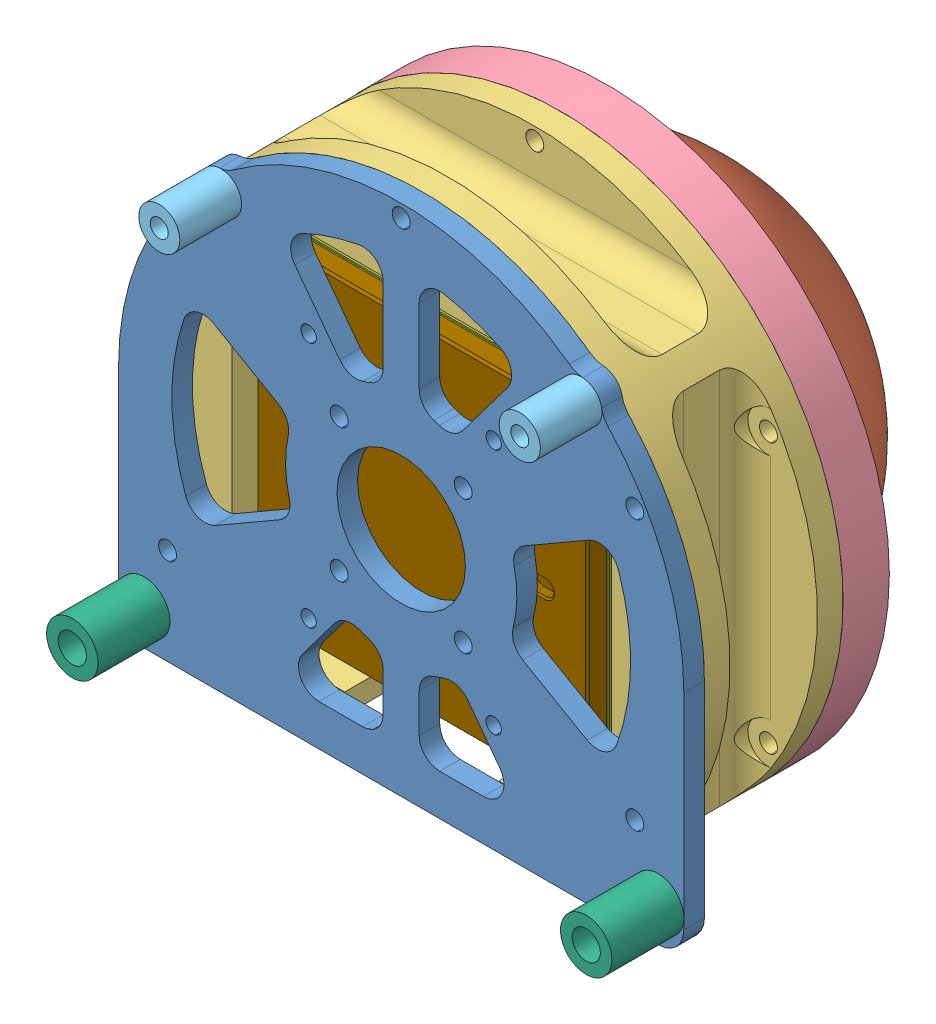
SolidWorks assembly MID保护安装版装配体, configuration 默认. Lengths in mm.
Overall size (1862.57 1865.26 855.73).
19 component instances, 15 part files, 20 mates.
Components (placement in the parent):
- IMU安装板11111-1: IMU安装板11111 [默认] at (-66.2823 -28.2156 -2) size (110 100 4)
- MID_360罩子-1: MID_360罩子 [默认] at (-66.2823 19.7844 -29) x (0.511073 -0.859537 0) z (0.859537 0.511073 0) size (99.6 45 99.6)
- MID保护罩支撑2222-1: MID保护罩支撑2222 [默认] at (-66.2823 -28.2156 -29) size (110 95.89 27)
- 舱盖固定环-1: 舱盖固定环 [默认] at (-66.2823 19.7844 -29) x (-1 0 0) z (0 0 -1) size (110 110 9)
- 支撑短-1: 支撑短 [默认] at (-31.2083 59.0344 2) x (-0.318059 -0.948071 0) z (0 0 1) size (8 8 12)
- 支撑长-1: 支撑长 [默认] at (-16.2823 -18.2156 2) x (-0.53223 0.8466 0) z (0 0 1) size (10 10 14)
- 支撑短-2: 支撑短 [默认] at (-101.3564 59.0344 2) x (0.71117 0.70302 0) z (0 0 1) size (8 8 12)
- 支撑长-2: 支撑长 [默认] at (-116.2823 -18.2156 2) x (0.671555 -0.740955 0) z (0 0 1) size (10 10 14)
- mid-360-fov-asm (1)-1: mid-360-fov-asm (1) [默认] at (-66.2823 19.7844 -27.9171) x (0 -1 0) z (1 0 0) size (1865.26 855.73 1862.57)
  - MID-360_4_ASM_2_ASM-1: MID-360_4_ASM_2_ASM [默认] at origin size (72.74 69.7 66.83)
    - MID-360_4_ASM_2_ASM-1: MID-360_4_ASM_2_ASM [默认] at origin size (71.74 36.3 66.83)
    - MID-360_4_1_1-1: MID-360_4_1_1 [默认] at origin size (52.18 60.17 55.44)
    - MID-360_4_2_1-1: MID-360_4_2_1 [默认] at origin size (64.79 8.1 64.79)
    - MID-360_4_3_2-1: MID-360_4_3_2 [默认] at origin size (13.8 16 22)
    - MID-360_4_4_1-1: MID-360_4_4_1 [默认] at origin size (0.41 0.13 0.13)
    - MID-360_4_5_1-1: MID-360_4_5_1 [默认] at origin size (0.41 0.13 0.13)
    - MID-360_4_6_1-1: MID-360_4_6_1 [默认] at origin size (0.41 0.13 0.13)
    - MID-360_4_7_1-1: MID-360_4_7_1 [默认] at origin size (0.41 0.13 0.13)
  - RECEIVE_FOV_MOVE_2-1: RECEIVE_FOV_MOVE_2 [默认] at origin size (1865.26 855.73 1862.57) (hidden)
Mates (geometry in assembly coordinates):
- 重合1: coincident anti-aligned: plane of IMU安装板11111-1 through (-66.2823 -28.2156 2) normal (0 0 1); plane of 支撑短-1 through (-31.2083 59.0344 2) normal (0 0 -1)
- 重合2: coincident anti-aligned: plane of IMU安装板11111-1 through (-66.2823 -28.2156 2) normal (0 0 1); plane of 支撑长-1 through (-16.2823 -18.2156 2) normal (0 0 -1)
- 重合3: coincident anti-aligned: plane of IMU安装板11111-1 through (-66.2823 -28.2156 2) normal (0 0 1); plane of 支撑长-2 through (-116.2823 -18.2156 2) normal (0 0 -1)
- 重合4: coincident anti-aligned: plane of IMU安装板11111-1 through (-66.2823 -28.2156 2) normal (0 0 1); plane of 支撑短-2 through (-101.3564 59.0344 2) normal (0 0 -1)
- 重合5: coincident anti-aligned: plane of IMU安装板11111-1 through (-66.2823 -28.2156 -2) normal (0 0 -1); plane of MID保护罩支撑2222-1 through (-66.2823 -28.2156 -2) normal (0 0 1)
- 同心10: concentric anti-aligned: cylinder of MID_360罩子-1 through (-66.2823 19.7844 -74) axis (0 0 -1) radius 49.8; cylinder of 舱盖固定环-1 through (-66.2823 19.7844 -29) axis (0 0 1) radius 49.8
- 重合6: coincident anti-aligned: plane of MID_360罩子-1 through (-89.1382 58.224 -34) normal (0 0 -1); plane of 舱盖固定环-1 through (-19.4516 19.7844 -34) normal (0 0 1)
- 同心11: concentric anti-aligned: cylinder of MID保护罩支撑2222-1 through (-66.2823 19.7844 -7) axis (0 0 -1) radius 55; cylinder of 舱盖固定环-1 through (-66.2823 19.7844 -38) axis (0 0 1) radius 55
- 重合7: coincident anti-aligned: plane of MID保护罩支撑2222-1 through (-66.2823 -28.2156 -29) normal (0 0 -1); plane of 舱盖固定环-1 through (-66.2823 19.7844 -29) normal (0 0 1)
- 重合8: coincident anti-aligned: plane of IMU安装板11111-1 through (-66.2823 -28.2156 -2) normal (0 0 -1); plane of mid-360-fov-asm (1)-1/MID-360_4_ASM_2_ASM-1/MID-360_4_2_1-1 through (-66.2823 19.7844 -2) normal (0 0 1)
- 同心12: concentric anti-aligned: cylinder of IMU安装板11111-1 through (-16.2823 -18.2156 -8) axis (0 0 1) radius 2.75; cylinder of 支撑长-1 through (-16.2823 -18.2156 16) axis (0 0 -1) radius 5
- 同心13: concentric anti-aligned: cylinder of IMU安装板11111-1 through (-116.2823 -18.2156 -8) axis (0 0 1) radius 2.75; cylinder of 支撑长-2 through (-116.2823 -18.2156 16) axis (0 0 -1) radius 5
- 同心14: concentric anti-aligned: cylinder of IMU安装板11111-1 through (-31.2083 59.0344 -8) axis (0 0 1) radius 1.75; cylinder of 支撑短-1 through (-31.2083 59.0344 14) axis (0 0 -1) radius 4
- 同心15: concentric aligned: cylinder of IMU安装板11111-1 through (-101.3564 59.0344 2) axis (0 0 -1) radius 4; cylinder of 支撑短-2 through (-101.3564 59.0344 14) axis (0 0 -1) radius 4
- 同心16: concentric anti-aligned: cylinder of IMU安装板11111-1 through (-116.2823 -18.2156 -8) axis (0 0 1) radius 2.75; cylinder of 支撑长-2 through (-116.2823 -18.2156 16) axis (0 0 -1) radius 5
- 同心17: concentric anti-aligned: cylinder of IMU安装板11111-1 through (-111.7487 -6.4656 -8) axis (0 0 1) radius 1.75; cylinder of MID保护罩支撑2222-1 through (-111.7487 -6.4656 -2) axis (0 0 -1) radius 1.75
- 同心18: concentric anti-aligned: cylinder of IMU安装板11111-1 through (-111.7487 46.0344 -8) axis (0 0 1) radius 1.75; cylinder of MID保护罩支撑2222-1 through (-111.7487 46.0344 -2) axis (0 0 -1) radius 1.75
- 同心19: concentric aligned: cylinder of IMU安装板11111-1 through (-84.2823 -4.2156 -8) axis (0 0 1) radius 1.5; cylinder of mid-360-fov-asm (1)-1/MID-360_4_ASM_2_ASM-1/MID-360_4_2_1-1 through (-84.2823 -4.2156 -7.096) axis (0 0 1) radius 1.25
- 同心20: concentric aligned: cylinder of IMU安装板11111-1 through (-48.2823 -4.2156 -8) axis (0 0 1) radius 1.5; cylinder of mid-360-fov-asm (1)-1/MID-360_4_ASM_2_ASM-1/MID-360_4_2_1-1 through (-48.2823 -4.2156 -7.096) axis (0 0 1) radius 1.25
- 同心21: concentric aligned: cylinder of MID保护罩支撑2222-1 through (-20.816 -6.4656 -2) axis (0 0 -1) radius 1.75; cylinder of 舱盖固定环-1 through (-20.816 -6.4656 -29) axis (0 0 -1) radius 1.75
